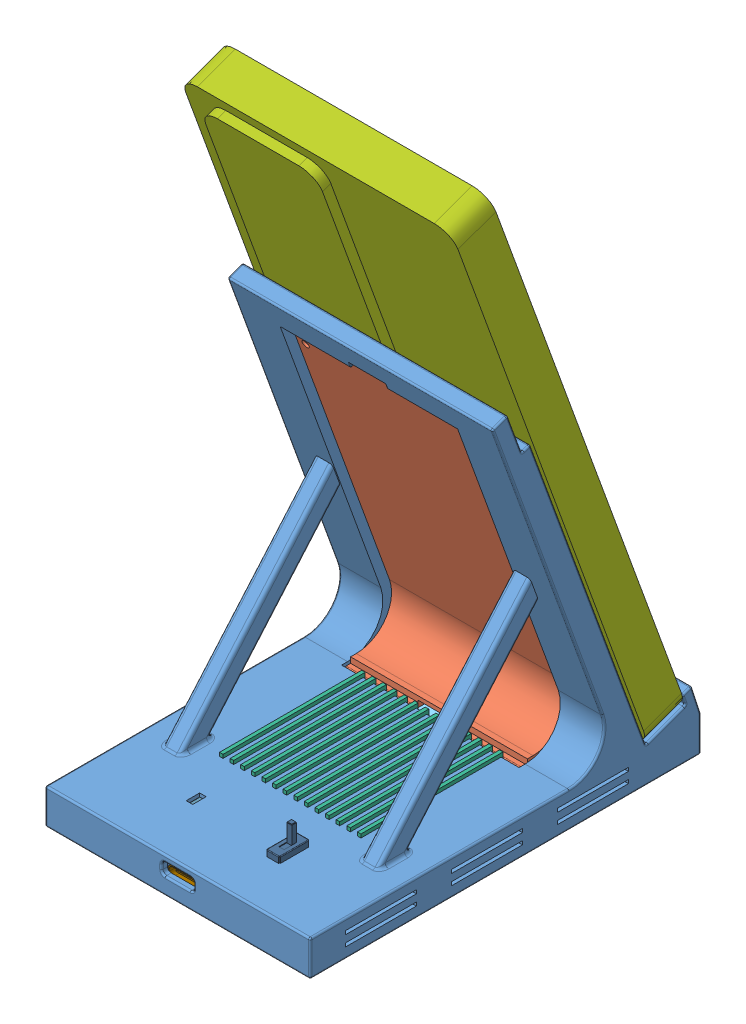
SolidWorks assembly P60支架装配体, configuration 默认. Lengths in mm.
Overall size (77 167.54 111.5).
30 component instances, 15 part files, 20 mates.
Components (placement in the parent):
- P60支架-1: P60支架 [默认] at (-19.3867 -35.6954 110) size (75 110.1 110.5)
- P60线圈支架零件-1: P60线圈支架零件 [默认] at (-19.3867 -31.7451 120.1792) x (0 0 -1) z (1 0 0) size (32.03 95.56 50)
- 充电线圈-1: 充电线圈 [默认] at (-19.3867 43.7507 97.2983) x (1 0 0) z (0 -0.939693 -0.34202) size (43 1.52 55.03)
- 充电零件板-1: 充电零件板 [默认] at (-19.3867 -29.6954 114.2678) x (1 0 0) z (0 0 -1) size (21 2 28)
- P60底板-1: P60底板 [默认] at (-34.8284 -35.6954 107.1856) x (0 0 -1) z (1 0 0) size (102.06 4.25 64.8)
- 散热器-1: 散热器 [默认] at (-19.3867 -29.6954 113.06) size (40 5 40.2)
- P60手机-1: P60手机 [默认] at (-19.3867 51.1245 97.9601) x (-1 0 0) z (0 0.34202 -0.939693) size (77 163.5 13.9)
- TypeC电路板-2: TypeC电路板 [默认] at (-41.3838 -27.6954 166.4715) x (0 0 -1) z (0 -1 0) size (30 34.97 13.16)
  - TypeC电路板.STEP-1: TypeC电路板.STEP [默认] at origin size (30 34.97 13.16)
    - TypeC______.STEP.STEP-1: TypeC______.STEP.STEP [默认] at origin size (30 34.97 13.16)
      - 5v06-R1.STEP.STEP-1: 5v06-R1.STEP.STEP [默认] at (25.0953 30.8357 1.2) x (-1 0 0) z (0 0 1) size (2 1.3 0.61)
        - R0805.STEP.STEP-1: R0805.STEP.STEP [默认] at origin size (2 1.3 0.61)
          - COMPOUND.STEP.STEP-1: COMPOUND.STEP.STEP [默认] at origin size (2 1.3 0.61)
      - 5v06-USB1.STEP.STEP-1: 5v06-USB1.STEP.STEP [默认] at (8.1992 21.9972 1.2) x (0 -1 0) z (0 0 1) size (8.95 7.58 4.16)
        - USB-C-SMD_TYPE-C-6PIN-2MD-073.STEP.STEP-1: USB-C-SMD_TYPE-C-6PIN-2MD-073.STEP.STEP [默认] at origin size (8.95 7.58 4.16)
          - COMPOUND-1.STEP.STEP-1: COMPOUND-1.STEP.STEP [默认] at origin size (8.95 7.58 4.16)
      - 5v06-U2.STEP.STEP-1: 5v06-U2.STEP.STEP [默认] at (19.685 34.9251 0) x (-1 0 0) z (0 0 -1) size (8.51 3.81 11.5)
        - SW-TH_DEALON_SS-12D01-GX.STEP.STEP-1: SW-TH_DEALON_SS-12D01-GX.STEP.STEP [默认] at origin size (8.51 3.81 11.5)
          - COMPOUND-2.STEP.STEP-1: COMPOUND-2.STEP.STEP [默认] at origin size (8.51 3.81 11.5)
      - 5v06-C1.STEP.STEP-1: 5v06-C1.STEP.STEP [默认] at (18.2118 28.8799 1.2) size (3.2 2.52 0.9)
        - C1210.STEP.STEP-1: C1210.STEP.STEP [默认] at origin size (3.2 2.52 0.9)
          - SOLID-3.STEP.STEP-1: SOLID-3.STEP.STEP [默认] at origin size (3.2 2.52 0.9)
      - 5v06-C2.STEP.STEP-1: 5v06-C2.STEP.STEP [默认] at (24.13 13.843 1.2) x (0 1 0) z (0 0 1) size (1.6 0.8 0.8)
        - C0603.STEP.STEP-1: C0603.STEP.STEP [默认] at origin size (1.6 0.8 0.8)
          - SOLID-4.STEP.STEP-1: SOLID-4.STEP.STEP [默认] at origin size (1.6 0.8 0.8)
      - 5v06-U4.STEP.STEP-1: 5v06-U4.STEP.STEP [默认] at (18.386 14.645 1.2) size (4.1 4.3 1.61)
        - SOT-89-3_L4.5-W2.5-P1.50-LS4.2-BR.STEP.STEP-1: SOT-89-3_L4.5-W2.5-P1.50-LS4.2-BR.STEP.STEP [默认] at origin size (4.1 4.3 1.61)
          - SOLID-5.STEP.STEP-1: SOLID-5.STEP.STEP [默认] at origin size (4.1 4.3 1.61)
      - Board.STEP.STEP-1: Board.STEP.STEP [默认] at origin size (29.97 34.97 1.2)
- Led5mmRojo_.step-1: Led5mmRojo_.step [默认] at (-19.3867 -30.6954 79) x (0 0 -1) z (1 0 0) size (25.5 5.8 5.4)
Mates (geometry in assembly coordinates):
- 重合8: coincident anti-aligned: plane of P60线圈支架零件-1 through (-19.3867 43.2377 98.7078) normal (0 0.34202 -0.939693); plane of 充电线圈-1 through (-19.3867 43.2377 98.7078) normal (0 -0.34202 0.939693)
- 同心1: concentric aligned: cylinder of P60线圈支架零件-1 through (-19.3867 43.2377 98.7078) axis (0 0.34202 -0.939693) radius 22; cylinder of 充电线圈-1 through (-19.3867 43.2377 98.7078) axis (0 0.34202 -0.939693) radius 21.5
- 重合15: coincident aligned: plane of P60线圈支架零件-1 through (-19.3867 -31.7451 120.1792) normal (1 0 0); plane of 充电线圈-1 through (-19.3867 43.7507 97.2983) normal (1 0 0)
- 宽度8: width aligned: plane of P60支架-1 through (18.1133 -25.6954 165) normal (1 0 0); plane of 散热器-1 through (-56.8867 -25.6954 165) normal (-1 0 0); plane of P60支架-1 through (0.6133 -27.6954 92.96) normal (1 0 0); plane of 散热器-1 through (-39.3867 -27.6954 92.96) normal (-1 0 0)
- 距离4: distance = 31.84 mm aligned: plane of 散热器-1 through (-39.3867 -27.6954 133.16) normal (0 0 1); plane of P60支架-1 through (-56.8867 -25.6954 165) normal (0 0 1)
- 重合43: coincident anti-aligned: plane of 充电零件板-1 through (-21.3867 -29.6954 108.6428) normal (0 1 0); plane of 散热器-1 through (-19.3867 -29.6954 113.06) normal (0 -1 0)
- 宽度9: width aligned: plane of 散热器-1 through (-39.3867 -27.6954 92.96) normal (-1 0 0); plane of 散热器-1 through (0.6133 -27.6954 92.96) normal (1 0 0); plane of 充电零件板-1 through (-29.8867 -31.6954 125.2678) normal (-1 0 0); plane of 充电零件板-1 through (-8.8867 -31.6954 125.2678) normal (1 0 0)
- 重合44: coincident aligned: plane of P60支架-1 through (-19.3867 -35.6954 110) normal (0 -1 0); plane of 底板-1 through (-34.8284 -35.6954 107.1856) normal (0 -1 0)
- 宽度11: width anti-aligned: plane of P60支架-1 through (-400019.3867 -35.6964 159) normal (0 0 -1); plane of P60底板-1 through (-400019.3867 -35.6964 61) normal (0 0 1); plane of P60支架-1 through (-51.1801 -34.1954 158.9) normal (0 0 1); plane of P60底板-1 through (-51.1801 -34.1954 61.1) normal (0 0 -1)
- 重合50: coincident anti-aligned: plane of P60支架-1 through (128.1581 75.4007 106.796) normal (0 0.34202 -0.939693); plane of P60手机-1 through (-19.3867 51.1245 97.9601) normal (0 -0.34202 0.939693)
- 重合51: coincident anti-aligned: plane of P60支架-1 through (-80.5764 -25.6954 70) normal (0 0.939693 0.34202); plane of P60手机-1 through (19.1133 -21.7964 59.2875) normal (0 -0.939693 -0.34202)
- 宽度14: width aligned: plane of P60手机-1 through (19.1133 131.8434 115.2078) normal (1 0 0); plane of P60支架-1 through (-57.8867 131.8434 115.2078) normal (-1 0 0); plane of P60手机-1 through (18.1133 -25.6954 165) normal (1 0 0); plane of P60支架-1 through (-56.8867 -25.6954 165) normal (-1 0 0)
- 距离9: distance = 0.1 mm anti-aligned: plane of TypeC电路板-2/TypeC电路板.STEP-1/TypeC______.STEP.STEP-1/Board.STEP.STEP-1 through (-1.8994 -27.6954 133.26) normal (0 0 -1); plane of 散热器-1 through (-39.3867 -27.6954 133.16) normal (0 0 1)
- 宽度15: width aligned: plane of P60支架-1 through (13.1133 -35.6964 291654.25) normal (-1 0 0); plane of P60支架-1 through (-51.8867 -35.6964 291654.25) normal (1 0 0); plane of TypeC电路板-2/TypeC电路板.STEP-1/TypeC______.STEP.STEP-1/Board.STEP.STEP-1 through (-36.874 -27.6954 133.26) normal (-1 0 0); plane of TypeC电路板-2/TypeC电路板.STEP-1/TypeC______.STEP.STEP-1/Board.STEP.STEP-1 through (-1.8994 -27.6954 155.7346) normal (1 0 0)
- 宽度16: width: plane of P60支架-1 through (-19.3867 -35.6954 110) normal (0 -1 0); plane of Led5mmRojo_.step-1 through (-19.3867 -25.6954 110) normal (0 1 0); cylinder of P60支架-1 through (-19.3867 -30.6954 61) axis (0 0 -1) radius 2.5
- 宽度17: width: plane of P60支架-1 through (18.1133 -25.6954 165) normal (1 0 0); plane of Led5mmRojo_.step-1 through (-56.8867 -25.6954 165) normal (-1 0 0); cylinder of P60支架-1 through (-19.3867 -30.6954 61) axis (0 0 -1) radius 2.5
- 平行1: parallel aligned: plane of P60支架-1 through (-19.3867 -35.6954 110) normal (0 -1 0); plane of Led5mmRojo_.step-1 through (-18.3667 -30.9454 62) normal (0 -1 0)
- 重合55: coincident anti-aligned: plane of P60支架-1 through (-400019.3867 -35.6964 61) normal (0 0 1); plane of Led5mmRojo_.step-1 through (-19.1867 -30.6954 61) normal (0 0 -1)
- 重合56: coincident anti-aligned: plane of P60支架-1 through (-19.3867 -27.6954 110) normal (0 -1 0); plane of TypeC电路板-2/TypeC电路板.STEP-1/TypeC______.STEP.STEP-1/Board.STEP.STEP-1 through (-19.3867 -27.6954 146.9186) normal (0 1 0)
- 重合57: coincident anti-aligned: plane of P60支架-1 through (-19.3867 -27.6954 110) normal (0 -1 0); plane of 散热器-1 through (-19.3867 -27.6954 113.06) normal (0 1 0)
